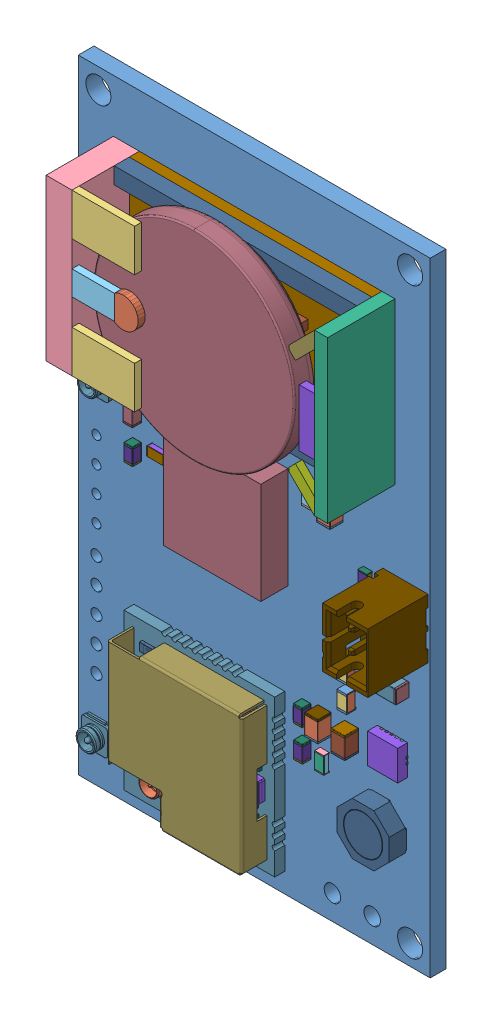
SolidWorks assembly Печатная плата Peggy Tracker, configuration По умолчанию. Lengths in mm.
Overall size (35 62 10.1).
297 component instances, 77 part files, 0 mates.
Components (placement in the parent):
- Печатная плата Peggy Tracker.step-1: Печатная плата Peggy Tracker.step [Default] at origin size (35 62 10.1)
  - Board.step-1: Board.step [Default] at origin size (35 62 1.56)
    - Open CASCADE STEP translator 6.8 1.1.1.step-1: Open CASCADE STEP translator 6.8 1.1.1.step [Default] at (0 0 -1.5596) size (35 62 1.56)
  - X1.step-1: X1.step [Default] at origin size (28 20 6.7)
    - 6517451856.step-1: 6517451856.step [Default] at (11.15 51.75 6) size (3 3 0.7)
      - Extruded.step-1: Extruded.step [Default] at origin size (3 3 0.7)
    - 6517450176.step-1: 6517450176.step [Default] at (9.1815 45.8445 6) size (6.22 4.19 0.7)
      - Extruded-0.step-1: Extruded-0.step [Default] at origin size (6.22 4.19 0.7)
    - 6517450176.step-2: 6517450176.step [Default] at (9.1815 57.6545 6) size (6.22 4.19 0.7)
      - Extruded-0.step-1: Extruded-0.step [Default] at origin size (6.22 4.19 0.7)
    - 6517449536.step-1: 6517449536.step [Default] at (4.785 51.7495 0) size (2.57 16 6.7)
      - Extruded-1.step-1: Extruded-1.step [Default] at origin size (2.57 16 6.7)
    - 6517449376.step-1: 6517449376.step [Default] at (8.1819 51.7635 6) size (4.22 2.41 0.7)
      - Extruded-2.step-1: Extruded-2.step [Default] at origin size (4.22 2.41 0.7)
    - 6517449056.step-1: 6517449056.step [Default] at (30.8492 51.7495 0) size (1.3 16 6.7)
      - Extruded-3.step-1: Extruded-3.step [Default] at origin size (1.3 16 6.7)
    - 6517448576.step-1: 6517448576.step [Default] at (28.9305 45.5257 6) size (2.54 3.55 0.7)
      - Extruded-4.step-1: Extruded-4.step [Default] at origin size (2.54 3.55 0.7)
    - 6517448256.step-1: 6517448256.step [Default] at (29.4382 51.4325 6) size (1.52 5.71 0.7)
      - Extruded-5.step-1: Extruded-5.step [Default] at origin size (1.52 5.71 0.7)
    - 6517447856.step-1: 6517447856.step [Default] at (18.1354 51.7495 0) size (24.13 16 1)
      - Extruded-6.step-1: Extruded-6.step [Default] at origin size (24.13 16 1)
    - 6517447456.step-1: 6517447456.step [Default] at (18.135 58.925 0) size (24.13 1.65 2.5)
      - Extruded-7.step-1: Extruded-7.step [Default] at origin size (24.13 1.65 2.5)
    - 6517447456.step-2: 6517447456.step [Default] at (18.1356 44.5737 0) size (24.13 1.65 2.5)
      - Extruded-7.step-1: Extruded-7.step [Default] at origin size (24.13 1.65 2.5)
    - 6517447056.step-1: 6517447056.step [Default] at (19.0875 48.7663 0) size (9.53 0.89 2.5)
      - Extruded-8.step-1: Extruded-8.step [Default] at origin size (9.53 0.89 2.5)
    - 6517447056.step-2: 6517447056.step [Default] at (19.0875 54.2273 0) size (9.53 0.89 2.5)
      - Extruded-8.step-1: Extruded-8.step [Default] at origin size (9.53 0.89 2.5)
    - 6517446256.step-1: 6517446256.step [Default] at (28.9302 57.972 6) size (2.54 3.55 0.7)
      - Extruded-9.step-1: Extruded-9.step [Default] at origin size (2.54 3.55 0.7)
    - CircuitWorks-BATT_CR2032.step-1: CircuitWorks-BATT_CR2032.step [Default] at (17.5 51.75 6) x (1 0 0) z (0 1 0) size (20 3.2 20)
  - XW2.step-1: XW2.step [Default] at origin size (2.86 3.01 1.29)
    - IPX.step-1: IPX.step [Default] at (2.0669 38.1281 1.27) x (0 1 0) z (0 0 1) size (3.01 2.86 1.29)
  - XW1.step-1: XW1.step [Default] at origin size (2.86 3.01 1.29)
    - IPX.step-1: IPX.step [Default] at (1.9653 7.4677 1.27) x (0 1 0) z (0 0 1) size (3.01 2.86 1.29)
  - R6.step-1: R6.step [Default] at origin size (0.9 1.7 0.55)
    - 6482559680.step-1: 6482559680.step [Default] at (28.8001 34.2999 0) x (0 -1 0) z (0 0 1) size (1.7 0.9 0.55)
      - Terminal.step-1: Terminal.step [Default] at (-0.85 -0.45 0) size (0.1 0.9 0.55)
        - Open_CASCADE_STEP_translator_6.8_15.2.1.step-1: Open_CASCADE_STEP_translator_6.8_15.2.1.step [Default] at origin size (0.1 0.9 0.55)
      - Terminal.step-2: Terminal.step [Default] at (0.85 0.45 0) x (-1 0 0) z (0 0 1) size (0.1 0.9 0.55)
        - Open_CASCADE_STEP_translator_6.8_15.2.1.step-1: Open_CASCADE_STEP_translator_6.8_15.2.1.step [Default] at origin size (0.1 0.9 0.55)
      - Mid_Body.step-1: Mid_Body.step [Default] at (-0.85 -0.45 0) size (1.59 0.9 0.44)
      - Mark.step-1: Mark.step [Default] at (-0.75 -0.45 0.495) size (1.5 0.9 0.06)
  - X3.step-1: X3.step [Default] at origin size (4.5 5.9 9.4)
    - B2B-PH-K-S(LF)(SN)--3DModel-STEP-56544.step-1: B2B-PH-K-S(LF)(SN)--3DModel-STEP-56544.step [Default] at (32.5449 33.0001 3) x (0 -1 0) z (-1 0 0) size (5.9 9.4 4.5)
  - R5.step-1: R5.step [Default] at origin size (0.95 1.75 0.95)
    - 6482560720.step-1: 6482560720.step [Default] at (27.1578 23.3326 0) x (0 1 0) z (0 0 1) size (1.75 0.95 0.95)
      - Terminal-1.step-1: Terminal-1.step [Default] at (-0.875 -0.475 0) size (0.2 0.95 0.95)
        - Open_CASCADE_STEP_translator_6.8_12.2.1.step-1: Open_CASCADE_STEP_translator_6.8_12.2.1.step [Default] at origin size (0.2 0.95 0.95)
      - Terminal-1.step-2: Terminal-1.step [Default] at (0.875 0.475 0) x (-1 0 0) z (0 0 1) size (0.2 0.95 0.95)
        - Open_CASCADE_STEP_translator_6.8_12.2.1.step-1: Open_CASCADE_STEP_translator_6.8_12.2.1.step [Default] at origin size (0.2 0.95 0.95)
      - Mid_Body-10.step-1: Mid_Body-10.step [Default] at (-0.875 -0.475 0) size (1.56 0.95 0.76)
      - Mark-11.step-1: Mark-11.step [Default] at (-0.675 -0.475 0.855) size (1.35 0.95 0.1)
  - R4.step-1: R4.step [Default] at origin size (0.95 1.75 0.95)
    - 6482560720.step-1: 6482560720.step [Default] at (27.1578 25.8726 0) x (0 1 0) z (0 0 1) size (1.75 0.95 0.95)
      - Terminal-1.step-1: Terminal-1.step [Default] at (-0.875 -0.475 0) size (0.2 0.95 0.95)
        - Open_CASCADE_STEP_translator_6.8_12.2.1.step-1: Open_CASCADE_STEP_translator_6.8_12.2.1.step [Default] at origin size (0.2 0.95 0.95)
      - Terminal-1.step-2: Terminal-1.step [Default] at (0.875 0.475 0) x (-1 0 0) z (0 0 1) size (0.2 0.95 0.95)
        - Open_CASCADE_STEP_translator_6.8_12.2.1.step-1: Open_CASCADE_STEP_translator_6.8_12.2.1.step [Default] at origin size (0.2 0.95 0.95)
      - Mid_Body-10.step-1: Mid_Body-10.step [Default] at (-0.875 -0.475 0) size (1.56 0.95 0.76)
      - Mark-11.step-1: Mark-11.step [Default] at (-0.675 -0.475 0.855) size (1.35 0.95 0.1)
  - R3.step-1: R3.step [Default] at origin size (0.9 1.7 0.55)
    - 6482559680.step-1: 6482559680.step [Default] at (28.8001 31.7999 0) x (0 -1 0) z (0 0 1) size (1.7 0.9 0.55)
      - Terminal.step-1: Terminal.step [Default] at (-0.85 -0.45 0) size (0.1 0.9 0.55)
        - Open_CASCADE_STEP_translator_6.8_15.2.1.step-1: Open_CASCADE_STEP_translator_6.8_15.2.1.step [Default] at origin size (0.1 0.9 0.55)
      - Terminal.step-2: Terminal.step [Default] at (0.85 0.45 0) x (-1 0 0) z (0 0 1) size (0.1 0.9 0.55)
        - Open_CASCADE_STEP_translator_6.8_15.2.1.step-1: Open_CASCADE_STEP_translator_6.8_15.2.1.step [Default] at origin size (0.1 0.9 0.55)
      - Mid_Body.step-1: Mid_Body.step [Default] at (-0.85 -0.45 0) size (1.59 0.9 0.44)
      - Mark.step-1: Mark.step [Default] at (-0.75 -0.45 0.495) size (1.5 0.9 0.06)
  - R2.step-1: R2.step [Default] at origin size (0.9 1.7 0.55)
    - 6482559840.step-1: 6482559840.step [Default] at (24.5109 16.5497 0) x (0 1 0) z (0 0 1) size (1.7 0.9 0.55)
      - Terminal-2.step-1: Terminal-2.step [Default] at (-0.85 -0.45 0) size (0.1 0.9 0.55)
        - Open_CASCADE_STEP_translator_6.8_15.2.1-12.step-1: Open_CASCADE_STEP_translator_6.8_15.2.1-12.step [Default] at origin size (0.1 0.9 0.55)
      - Terminal-2.step-2: Terminal-2.step [Default] at (0.85 0.45 0) x (-1 0 0) z (0 0 1) size (0.1 0.9 0.55)
        - Open_CASCADE_STEP_translator_6.8_15.2.1-12.step-1: Open_CASCADE_STEP_translator_6.8_15.2.1-12.step [Default] at origin size (0.1 0.9 0.55)
      - Mid_Body-13.step-1: Mid_Body-13.step [Default] at (-0.85 -0.45 0) size (1.59 0.9 0.44)
      - Mark-14.step-1: Mark-14.step [Default] at (-0.75 -0.45 0.495) size (1.5 0.9 0.06)
  - R1.step-1: R1.step [Default] at origin size (1.7 0.9 0.55)
    - 6517452256.step-1: 6517452256.step [Default] at (8.2043 34.8489 0) size (1.7 0.9 0.55)
      - Terminal-3.step-1: Terminal-3.step [Default] at (-0.85 -0.45 0) size (0.1 0.9 0.55)
        - Open_CASCADE_STEP_translator_6.8_15.2.1-15.step-1: Open_CASCADE_STEP_translator_6.8_15.2.1-15.step [Default] at origin size (0.1 0.9 0.55)
      - Terminal-3.step-2: Terminal-3.step [Default] at (0.85 0.45 0) x (-1 0 0) z (0 0 1) size (0.1 0.9 0.55)
        - Open_CASCADE_STEP_translator_6.8_15.2.1-15.step-1: Open_CASCADE_STEP_translator_6.8_15.2.1-15.step [Default] at origin size (0.1 0.9 0.55)
      - Mid_Body-16.step-1: Mid_Body-16.step [Default] at (-0.85 -0.45 0) size (1.59 0.9 0.44)
      - Mark-17.step-1: Mark-17.step [Default] at (-0.75 -0.45 0.495) size (1.5 0.9 0.06)
  - L2.step-1: L2.step [Default] at origin size (5.2 5.2 1.8)
    - 6482573440.step-1: 6482573440.step [Default] at (30.1268 13.8076 0.2) x (1 0 0) z (0 -1 0) size (5.2 1.8 5.2)
  - L1.step-1: L1.step [Default] at origin size (0.95 1.75 0.95)
    - 6482561680.step-1: 6482561680.step [Default] at (5.85 37.366 0) x (0 1 0) z (0 0 1) size (1.75 0.95 0.95)
      - Terminal-4.step-1: Terminal-4.step [Default] at (-0.875 -0.475 0) size (1.75 0.95 0.95)
        - Open_CASCADE_STEP_translator_6.8_2.1.1.step-1: Open_CASCADE_STEP_translator_6.8_2.1.1.step [Default] at origin size (0.2 0.95 0.95)
        - Open_CASCADE_STEP_translator_6.8_2.1.2.step-1: Open_CASCADE_STEP_translator_6.8_2.1.2.step [Default] at origin size (0.2 0.95 0.95)
      - Mid_Body-18.step-1: Mid_Body-18.step [Default] at (-0.875 -0.475 0) size (1.35 0.95 0.95)
        - Open_CASCADE_STEP_translator_6.8_2.2.1.step-1: Open_CASCADE_STEP_translator_6.8_2.2.1.step [Default] at origin size (1.35 0.95 0.95)
  - DD2.step-1: DD2.step [Default] at origin size (15 15.5 3.52)
    - 3D_RAK3172.step-1: 3D_RAK3172.step [Default] at (20.536 20.4601 1) x (-1 0 0) z (0 0 1) size (15 15.5 3.52)
      - Board-1.step-1: Board-1.step [Default] at origin size (15 15.5 1.01)
        - Open_CASCADE_STEP_translator_6.8_1.1.1.step-1: Open_CASCADE_STEP_translator_6.8_1.1.1.step [Default] at (0 0 -1.014) size (15 15.5 1.01)
          - Open_CASCADE_STEP_translator_6.8_1.1.1.1.step-1: Open_CASCADE_STEP_translator_6.8_1.1.1.1.step [Default] at origin size (15 15.5 1.01)
      - R11.step-1: R11.step [Default] at origin size (0.6 0.3 0.3)
        - 0201_SMD_Capacitor.step-1: 0201_SMD_Capacitor.step [Default] at (3.4751 6.9342 0.2794) x (-1 0 0) z (0 0 1) size (0.6 0.3 0.3)
      - U2.step-1: U2.step [Default] at origin size (0.99 1.02 0.75)
        - 6590464912.step-1: 6590464912.step [Default] at (5.4483 13.05 0) size (0.99 1.02 0.75)
          - Extruded-19.step-1: Extruded-19.step [Default] at origin size (0.99 1.02 0.75)
      - R4-1.step-1: R4-1.step [Default] at origin size (0.68 0.33 0.34)
        - R0201.step-1: R0201.step [Default] at (3.9176 5.9192 0) x (1 0 0) z (0 -1 0) size (0.68 0.34 0.33)
      - R3-1.step-1: R3-1.step [Default] at origin size (0.33 0.68 0.34)
        - R0201.step-1: R0201.step [Default] at (4.1676 5.6692 0) x (0 1 0) z (1 0 0) size (0.68 0.34 0.33)
      - L2-1.step-1: L2-1.step [Default] at origin size (1.15 0.55 0.41)
        - RES_1005-0402.step-1: RES_1005-0402.step [Default] at (2.2661 6.0198 0) x (1 0 0) z (0 -1 0) size (1.15 0.41 0.55)
      - C10.step-1: C10.step [Default] at origin size (0.6 0.3 0.3)
        - 0201_SMD_Capacitor.step-1: 0201_SMD_Capacitor.step [Default] at (7.1835 13.462 0.2794) x (-1 0 0) z (0 0 1) size (0.6 0.3 0.3)
      - C9.step-1: C9.step [Default] at origin size (0.6 0.3 0.3)
        - 0201_SMD_Capacitor.step-1: 0201_SMD_Capacitor.step [Default] at (7.1835 13.97 0.2794) x (-1 0 0) z (0 0 1) size (0.6 0.3 0.3)
      - C8.step-1: C8.step [Default] at origin size (0.6 0.3 0.3)
        - 0201_SMD_Capacitor.step-1: 0201_SMD_Capacitor.step [Default] at (7.1835 12.954 0.2794) x (-1 0 0) z (0 0 1) size (0.6 0.3 0.3)
      - C7.step-1: C7.step [Default] at origin size (0.6 0.3 0.3)
        - 0201_SMD_Capacitor.step-1: 0201_SMD_Capacitor.step [Default] at (6.0793 11.938 0.2794) x (1 0 0) z (0 0 1) size (0.6 0.3 0.3)
      - C6.step-1: C6.step [Default] at origin size (0.6 0.3 0.3)
        - 0201_SMD_Capacitor.step-1: 0201_SMD_Capacitor.step [Default] at (3.8855 13.5541 0.2794) x (-1 0 0) z (0 0 1) size (0.6 0.3 0.3)
      - CON1.step-1: CON1.step [Default] at origin size (3.4 3.1 1.25)
        - UFL-R-SMD.step-1: UFL-R-SMD.step [Default] at (11.3537 12.7757 0) x (1 0 0) z (0 0 1) size (3.4 3.1 1.25)
          - Part_525.step-1: Part_525.step [Default] at origin size (3 2.6 0.35)
          - Part_739.step-1: Part_739.step [Default] at origin size (2 2 0.9)
          - Part_578.step-1: Part_578.step [Default] at origin size (0.6 0.5 0.1)
          - Part_540.step-1: Part_540.step [Default] at origin size (0.4 1.8 0.1)
          - Part_562.step-1: Part_562.step [Default] at origin size (0.4 1.8 0.1)
          - Part_555.step-1: Part_555.step [Default] at origin size (0.6 0.5 0.1)
      - C4.step-1: C4.step [Default] at origin size (0.6 0.3 0.3)
        - 0201_SMD_Capacitor.step-1: 0201_SMD_Capacitor.step [Default] at (3.7799 9.398 0.2794) x (-1 0 0) z (0 0 1) size (0.6 0.3 0.3)
      - U1.step-1: U1.step [Default] at origin size (7.02 7.02 0.8)
        - QFN48_7x7.step-1: QFN48_7x7.step [Default] at (8.8366 6.9818 0) x (0 1 0) z (1 0 0) size (7.02 0.8 7.02)
      - X1-1.step-1: X1-1.step [Default] at origin size (1.61 2.01 0.71)
        - NT2016SA.step-1: NT2016SA.step [Default] at (1.7496 8.4946 0) x (0 1 0) z (1 0 0) size (2.01 0.71 1.61)
      - C43.step-1: C43.step [Default] at origin size (0.6 0.3 0.3)
        - 0201_SMD_Capacitor.step-1: 0201_SMD_Capacitor.step [Default] at (3.7799 9.9822 0.2794) x (-1 0 0) z (0 0 1) size (0.6 0.3 0.3)
      - C42.step-1: C42.step [Default] at origin size (0.3 0.6 0.3)
        - 0201_SMD_Capacitor.step-1: 0201_SMD_Capacitor.step [Default] at (3.0734 7.9709 0.2794) x (0 -1 0) z (0 0 1) size (0.6 0.3 0.3)
      - R9.step-1: R9.step [Default] at origin size (0.6 0.3 0.3)
        - 0201_SMD_Capacitor.step-1: 0201_SMD_Capacitor.step [Default] at (3.7799 8.8138 0.2794) x (-1 0 0) z (0 0 1) size (0.6 0.3 0.3)
      - C1.step-1: C1.step [Default] at origin size (0.6 0.3 0.3)
        - 0201_SMD_Capacitor.step-1: 0201_SMD_Capacitor.step [Default] at (7.0445 11.557 0.2794) x (1 0 0) z (0 0 1) size (0.6 0.3 0.3)
      - C2.step-1: C2.step [Default] at origin size (0.3 0.6 0.3)
        - 0201_SMD_Capacitor.step-1: 0201_SMD_Capacitor.step [Default] at (7.9756 12.2635 0.2794) x (0 -1 0) z (0 0 1) size (0.6 0.3 0.3)
      - C3.step-1: C3.step [Default] at origin size (0.3 0.6 0.3)
        - 0201_SMD_Capacitor.step-1: 0201_SMD_Capacitor.step [Default] at (2.1844 13.4518 0.2794) x (0 -1 0) z (0 0 1) size (0.6 0.3 0.3)
      - C11.step-1: C11.step [Default] at origin size (0.6 0.3 0.3)
        - 0201_SMD_Capacitor.step-1: 0201_SMD_Capacitor.step [Default] at (1.6623 11.9866 0.2794) x (1 0 0) z (0 0 1) size (0.6 0.3 0.3)
      - C12.step-1: C12.step [Default] at origin size (0.6 0.3 0.3)
        - 0201_SMD_Capacitor.step-1: 0201_SMD_Capacitor.step [Default] at (3.2813 12.573 0.2794) x (1 0 0) z (0 0 1) size (0.6 0.3 0.3)
      - C13.step-1: C13.step [Default] at origin size (0.3 0.6 0.3)
        - 0201_SMD_Capacitor.step-1: 0201_SMD_Capacitor.step [Default] at (4.4958 12.0697 0.2794) x (0 1 0) z (0 0 1) size (0.6 0.3 0.3)
      - C14.step-1: C14.step [Default] at origin size (0.3 0.6 0.3)
        - 0201_SMD_Capacitor.step-1: 0201_SMD_Capacitor.step [Default] at (2.7178 12.6739 0.2794) x (0 -1 0) z (0 0 1) size (0.6 0.3 0.3)
      - C17.step-1: C17.step [Default] at origin size (0.3 0.6 0.3)
        - 0201_SMD_Capacitor.step-1: 0201_SMD_Capacitor.step [Default] at (7.6708 14.4693 0.2794) x (0 -1 0) z (0 0 1) size (0.6 0.3 0.3)
      - C18.step-1: C18.step [Default] at origin size (0.6 0.3 0.3)
        - 0201_SMD_Capacitor.step-1: 0201_SMD_Capacitor.step [Default] at (9.1901 14.1224 0.2794) x (-1 0 0) z (0 0 1) size (0.6 0.3 0.3)
      - C19.step-1: C19.step [Default] at origin size (0.3 0.6 0.3)
        - 0201_SMD_Capacitor.step-1: 0201_SMD_Capacitor.step [Default] at (2.8814 10.8799 0.2794) x (0 1 0) z (0 0 1) size (0.6 0.3 0.3)
      - C22.step-1: C22.step [Default] at origin size (0.3 0.6 0.3)
        - 0201_SMD_Capacitor.step-1: 0201_SMD_Capacitor.step [Default] at (2.0432 11.4801 0.2794) x (0 -1 0) z (0 0 1) size (0.6 0.3 0.3)
      - C21.step-1: C21.step [Default] at origin size (0.3 0.6 0.3)
        - 0201_SMD_Capacitor.step-1: 0201_SMD_Capacitor.step [Default] at (1.5606 11.4801 0.2794) x (0 -1 0) z (0 0 1) size (0.6 0.3 0.3)
      - C23.step-1: C23.step [Default] at origin size (1 0.5 0.5)
        - C0402.step-1: C0402.step [Default] at (8.9644 1.5539 0.254) x (1 0 0) z (0 0 1) size (1 0.5 0.5)
      - C24.step-1: C24.step [Default] at origin size (0.6 0.3 0.3)
        - 0201_SMD_Capacitor.step-1: 0201_SMD_Capacitor.step [Default] at (4.7197 3.8862 0.2794) x (-1 0 0) z (0 0 1) size (0.6 0.3 0.3)
      - C26.step-1: C26.step [Default] at origin size (0.3 0.6 0.3)
        - 0201_SMD_Capacitor.step-1: 0201_SMD_Capacitor.step [Default] at (10.541 2.2265 0.2794) x (0 -1 0) z (0 0 1) size (0.6 0.3 0.3)
      - C44.step-1: C44.step [Default] at origin size (0.6 0.3 0.3)
        - 0201_SMD_Capacitor.step-1: 0201_SMD_Capacitor.step [Default] at (4.7919 9.9822 0.2794) x (-1 0 0) z (0 0 1) size (0.6 0.3 0.3)
      - C29.step-1: C29.step [Default] at origin size (0.6 0.3 0.3)
        - 0201_SMD_Capacitor.step-1: 0201_SMD_Capacitor.step [Default] at (3.9925 7.8486 0.2794) x (1 0 0) z (0 0 1) size (0.6 0.3 0.3)
      - C25.step-1: C25.step [Default] at origin size (0.3 0.6 0.3)
        - 0201_SMD_Capacitor.step-1: 0201_SMD_Capacitor.step [Default] at (10.287 1.6263 0.2794) x (0 1 0) z (0 0 1) size (0.6 0.3 0.3)
      - C31.step-1: C31.step [Default] at origin size (0.6 0.3 0.3)
        - 0201_SMD_Capacitor.step-1: 0201_SMD_Capacitor.step [Default] at (3.9965 7.239 0.2794) x (1 0 0) z (0 0 1) size (0.6 0.3 0.3)
      - C32.step-1: C32.step [Default] at origin size (0.6 0.3 0.3)
        - 0201_SMD_Capacitor.step-1: 0201_SMD_Capacitor.step [Default] at (7.8533 2.3622 0.2794) x (1 0 0) z (0 0 1) size (0.6 0.3 0.3)
      - C33.step-1: C33.step [Default] at origin size (1 0.5 0.5)
        - C0402.step-1: C0402.step [Default] at (5.3048 2.0461 0.254) x (-1 0 0) z (0 0 1) size (1 0.5 0.5)
      - C34.step-1: C34.step [Default] at origin size (0.3 0.6 0.3)
        - 0201_SMD_Capacitor.step-1: 0201_SMD_Capacitor.step [Default] at (4.318 4.2211 0.2794) x (0 1 0) z (0 0 1) size (0.6 0.3 0.3)
      - C35.step-1: C35.step [Default] at origin size (0.6 0.3 0.3)
        - 0201_SMD_Capacitor.step-1: 0201_SMD_Capacitor.step [Default] at (9.0365 2.3622 0.2794) x (1 0 0) z (0 0 1) size (0.6 0.3 0.3)
      - C36.step-1: C36.step [Default] at origin size (0.3 0.6 0.3)
        - 0201_SMD_Capacitor.step-1: 0201_SMD_Capacitor.step [Default] at (13.0302 10.0751 0.2794) x (0 -1 0) z (0 0 1) size (0.6 0.3 0.3)
      - C37.step-1: C37.step [Default] at origin size (0.3 0.6 0.3)
        - 0201_SMD_Capacitor.step-1: 0201_SMD_Capacitor.step [Default] at (3.7338 4.2211 0.2794) x (0 1 0) z (0 0 1) size (0.6 0.3 0.3)
      - C38.step-1: C38.step [Default] at origin size (1 0.5 0.5)
        - C0402.step-1: C0402.step [Default] at (2.3114 4.7323 0.254) x (1 0 0) z (0 0 1) size (1 0.5 0.5)
      - C39.step-1: C39.step [Default] at origin size (0.6 0.3 0.3)
        - 0201_SMD_Capacitor.step-1: 0201_SMD_Capacitor.step [Default] at (4.0593 3.1881 0.2794) x (-1 0 0) z (0 0 1) size (0.6 0.3 0.3)
      - C40.step-1: C40.step [Default] at origin size (0.3 0.6 0.3)
        - 0201_SMD_Capacitor.step-1: 0201_SMD_Capacitor.step [Default] at (3.6576 1.7319 0.2794) x (0 1 0) z (0 0 1) size (0.6 0.3 0.3)
      - L1-1.step-1: L1-1.step [Default] at origin size (0.68 0.33 0.34)
        - R0201.step-1: R0201.step [Default] at (7.8526 11.2014 0) x (-1 0 0) z (0 1 0) size (0.68 0.34 0.33)
      - L3.step-1: L3.step [Default] at origin size (0.33 0.68 0.34)
        - R0201.step-1: R0201.step [Default] at (1.7272 13.1318 0) x (0 -1 0) z (-1 0 0) size (0.68 0.34 0.33)
      - L5.step-1: L5.step [Default] at origin size (0.68 0.33 0.34)
        - R0201.step-1: R0201.step [Default] at (8.0772 13.3096 0) x (-1 0 0) z (0 1 0) size (0.68 0.34 0.33)
      - L6.step-1: L6.step [Default] at origin size (1 0.5 0.5)
        - C0402.step-1: C0402.step [Default] at (5.822 11.0823 0.254) x (1 0 0) z (0 0 1) size (1 0.5 0.5)
      - L7.step-1: L7.step [Default] at origin size (0.68 0.33 0.34)
        - R0201.step-1: R0201.step [Default] at (3.5854 12.1158 0) x (1 0 0) z (0 -1 0) size (0.68 0.34 0.33)
      - L9.step-1: L9.step [Default] at origin size (1.15 0.55 0.41)
        - RES_1005-0402.step-1: RES_1005-0402.step [Default] at (3.9641 11.3538 0) x (-1 0 0) z (0 1 0) size (1.15 0.41 0.55)
      - L20.step-1: L20.step [Default] at origin size (1.6 0.8 0.3)
        - 6559637360.step-1: 6559637360.step [Default] at (12.3698 2.0828 0) x (-1 0 0) z (0 1 0) size (1.6 0.3 0.8)
      - L30.step-1: L30.step [Default] at origin size (1.15 0.55 0.41)
        - RES_1005-0402.step-1: RES_1005-0402.step [Default] at (7.1263 1.8 0) x (-1 0 0) z (0 1 0) size (1.15 0.41 0.55)
      - X2.step-1: X2.step [Default] at origin size (1.2 2 0.61)
        - crystal_rtf2012.step-1: crystal_rtf2012.step [Default] at (2.25 2.8402 0) x (0 1 0) z (1 0 0) size (2 0.61 1.2)
      - R2-1.step-1: R2-1.step [Default] at origin size (0.68 0.33 0.34)
        - R0201.step-1: R0201.step [Default] at (1.9613 10.1854 0) x (1 0 0) z (0 -1 0) size (0.68 0.34 0.33)
      - C5.step-1: C5.step [Default] at origin size (0.6 0.3 0.3)
        - 0201_SMD_Capacitor.step-1: 0201_SMD_Capacitor.step [Default] at (1.8749 6.9342 0.2794) x (-1 0 0) z (0 0 1) size (0.6 0.3 0.3)
      - Free-Models.step-1: Free-Models.step [Default] at origin size (13.4 13.9 2.5)
        - D030A-______.step-1: D030A-______.step [Default] at (2.429 -1.8288 0) size (13.4 13.9 2.5)
  - DD1.step-1: DD1.step [Default] at origin size (9.7 10.1 2.8)
    - 6482566000.step-1: 6482566000.step [Default] at (16.1 34.85 0) x (1 0 0) z (0 0 1) size (9.7 10.1 2.8)
      - Body.step-1: Body.step [Default] at (0 0 0.1) size (9.7 10.1 2.7)
      - Pins.step-1: Pins.step [Default] at origin size (9.56 9.36 0.1)
  - DA1.step-1: DA1.step [Default] at origin size (3 3 1)
    - 6482561360.step-1: 6482561360.step [Default] at (31.2728 20.6686 0) x (0 1 0) z (0 0 1) size (3 3 1)
      - FRAME-DRC0010J.step-1: FRAME-DRC0010J.step [Default] x (1 0 0) z (0 -1 0) size (3 0.2 3)
        - Open CASCADE STEP translator 6.8 1.16.1.2.1.step-1: Open CASCADE STEP translator 6.8 1.16.1.2.1.step [Default] at origin size (1.9 0.2 3)
        - Open CASCADE STEP translator 6.8 1.16.1.2.2.step-1: Open CASCADE STEP translator 6.8 1.16.1.2.2.step [Default] at origin size (0.4 0.2 0.24)
        - Open CASCADE STEP translator 6.8 1.16.1.2.3.step-1: Open CASCADE STEP translator 6.8 1.16.1.2.3.step [Default] at origin size (0.4 0.2 0.24)
        - Open CASCADE STEP translator 6.8 1.16.1.2.4.step-1: Open CASCADE STEP translator 6.8 1.16.1.2.4.step [Default] at origin size (0.4 0.2 0.24)
        - Open CASCADE STEP translator 6.8 1.16.1.2.5.step-1: Open CASCADE STEP translator 6.8 1.16.1.2.5.step [Default] at origin size (0.4 0.2 0.24)
        - Open CASCADE STEP translator 6.8 1.16.1.2.6.step-1: Open CASCADE STEP translator 6.8 1.16.1.2.6.step [Default] at origin size (0.4 0.2 0.24)
        - Open CASCADE STEP translator 6.8 1.16.1.2.7.step-1: Open CASCADE STEP translator 6.8 1.16.1.2.7.step [Default] at origin size (0.4 0.2 0.24)
        - Open CASCADE STEP translator 6.8 1.16.1.2.8.step-1: Open CASCADE STEP translator 6.8 1.16.1.2.8.step [Default] at origin size (0.4 0.2 0.24)
        - Open CASCADE STEP translator 6.8 1.16.1.2.9.step-1: Open CASCADE STEP translator 6.8 1.16.1.2.9.step [Default] at origin size (0.4 0.2 0.24)
        - Open CASCADE STEP translator 6.8 1.16.1.2.10.step-1: Open CASCADE STEP translator 6.8 1.16.1.2.10.step [Default] at origin size (0.4 0.2 0.24)
        - Open CASCADE STEP translator 6.8 1.16.1.2.11.step-1: Open CASCADE STEP translator 6.8 1.16.1.2.11.step [Default] at origin size (0.4 0.2 0.24)
      - BODY-SON.step-1: BODY-SON.step [Default] at (0 0 0.025) x (1 0 0) z (0 -1 0) size (3 0.97 3)
  - C8-1.step-1: C8-1.step [Default] at origin size (1.4 2.15 1.4)
    - 6482573680.step-1: 6482573680.step [Default] at (27.1929 19.9035 0) x (0 -1 0) z (0 0 1) size (2.15 1.4 1.4)
      - Terminal-5.step-1: Terminal-5.step [Default] at (-1.075 -0.7 0) size (2.15 1.4 1.4)
        - Open_CASCADE_STEP_translator_6.8_5.1.1.step-1: Open_CASCADE_STEP_translator_6.8_5.1.1.step [Default] at origin size (0.2 1.4 1.4)
        - Open_CASCADE_STEP_translator_6.8_5.1.2.step-1: Open_CASCADE_STEP_translator_6.8_5.1.2.step [Default] at origin size (0.2 1.4 1.4)
      - Mid_Body-1.step-1: Mid_Body-1.step [Default] at (-1.075 -0.7 0) size (1.75 1.4 1.4)
        - Open_CASCADE_STEP_translator_6.8_5.2.1.step-1: Open_CASCADE_STEP_translator_6.8_5.2.1.step [Default] at origin size (1.75 1.4 1.4)
  - C7-1.step-1: C7-1.step [Default] at origin size (2.1 1.35 1.35)
    - 6482573600.step-1: 6482573600.step [Default] at (31.889 26.8 0) x (1 0 0) z (0 0 1) size (2.1 1.35 1.35)
      - Terminal-6.step-1: Terminal-6.step [Default] at (-1.05 -0.675 0) size (2.1 1.35 1.35)
        - Open_CASCADE_STEP_translator_6.8_24.1.1.step-1: Open_CASCADE_STEP_translator_6.8_24.1.1.step [Default] at origin size (0.2 1.35 1.35)
        - Open_CASCADE_STEP_translator_6.8_24.1.2.step-1: Open_CASCADE_STEP_translator_6.8_24.1.2.step [Default] at origin size (0.2 1.35 1.35)
      - Mid_Body-2.step-1: Mid_Body-2.step [Default] at (-1.05 -0.675 0) size (1.7 1.35 1.35)
        - Open_CASCADE_STEP_translator_6.8_24.2.1.step-1: Open_CASCADE_STEP_translator_6.8_24.2.1.step [Default] at origin size (1.7 1.35 1.35)
  - C6-1.step-1: C6-1.step [Default] at origin size (0.9 1.7 0.9)
    - 6482559520.step-1: 6482559520.step [Default] at (22.727 16.763 0) x (0 -1 0) z (0 0 1) size (1.7 0.9 0.9)
      - Terminal-7.step-1: Terminal-7.step [Default] at (-0.85 -0.45 0) size (1.7 0.9 0.9)
        - Open_CASCADE_STEP_translator_6.8_5.1.1-20.step-1: Open_CASCADE_STEP_translator_6.8_5.1.1-20.step [Default] at origin size (0.2 0.9 0.9)
        - Open_CASCADE_STEP_translator_6.8_5.1.2-21.step-1: Open_CASCADE_STEP_translator_6.8_5.1.2-21.step [Default] at origin size (0.2 0.9 0.9)
      - Mid_Body-3.step-1: Mid_Body-3.step [Default] at (-0.85 -0.45 0) size (1.3 0.9 0.9)
        - Open_CASCADE_STEP_translator_6.8_5.2.1-22.step-1: Open_CASCADE_STEP_translator_6.8_5.2.1-22.step [Default] at origin size (1.3 0.9 0.9)
  - C5-1.step-1: C5-1.step [Default] at origin size (1.35 2.1 1.35)
    - 6482568960.step-1: 6482568960.step [Default] at (24.505 19.939 0) x (0 -1 0) z (0 0 1) size (2.1 1.35 1.35)
      - Terminal-8.step-1: Terminal-8.step [Default] at (-1.05 -0.675 0) size (2.1 1.35 1.35)
        - Open_CASCADE_STEP_translator_6.8_24.1.1-23.step-1: Open_CASCADE_STEP_translator_6.8_24.1.1-23.step [Default] at origin size (0.2 1.35 1.35)
        - Open_CASCADE_STEP_translator_6.8_24.1.2-24.step-1: Open_CASCADE_STEP_translator_6.8_24.1.2-24.step [Default] at origin size (0.2 1.35 1.35)
      - Mid_Body-4.step-1: Mid_Body-4.step [Default] at (-1.05 -0.675 0) size (1.7 1.35 1.35)
        - Open_CASCADE_STEP_translator_6.8_24.2.1-25.step-1: Open_CASCADE_STEP_translator_6.8_24.2.1-25.step [Default] at origin size (1.7 1.35 1.35)
  - C4-1.step-1: C4-1.step [Default] at origin size (0.9 1.7 0.9)
    - 6482559520.step-1: 6482559520.step [Default] at (22.7 19.888 0) x (0 -1 0) z (0 0 1) size (1.7 0.9 0.9)
      - Terminal-7.step-1: Terminal-7.step [Default] at (-0.85 -0.45 0) size (1.7 0.9 0.9)
        - Open_CASCADE_STEP_translator_6.8_5.1.1-20.step-1: Open_CASCADE_STEP_translator_6.8_5.1.1-20.step [Default] at origin size (0.2 0.9 0.9)
        - Open_CASCADE_STEP_translator_6.8_5.1.2-21.step-1: Open_CASCADE_STEP_translator_6.8_5.1.2-21.step [Default] at origin size (0.2 0.9 0.9)
      - Mid_Body-3.step-1: Mid_Body-3.step [Default] at (-0.85 -0.45 0) size (1.3 0.9 0.9)
        - Open_CASCADE_STEP_translator_6.8_5.2.1-22.step-1: Open_CASCADE_STEP_translator_6.8_5.2.1-22.step [Default] at origin size (1.3 0.9 0.9)
  - C3-1.step-1: C3-1.step [Default] at origin size (1.35 2.1 1.35)
    - 6482568960.step-1: 6482568960.step [Default] at (25.7048 39.0008 0) x (0 -1 0) z (0 0 1) size (2.1 1.35 1.35)
      - Terminal-8.step-1: Terminal-8.step [Default] at (-1.05 -0.675 0) size (2.1 1.35 1.35)
        - Open_CASCADE_STEP_translator_6.8_24.1.1-23.step-1: Open_CASCADE_STEP_translator_6.8_24.1.1-23.step [Default] at origin size (0.2 1.35 1.35)
        - Open_CASCADE_STEP_translator_6.8_24.1.2-24.step-1: Open_CASCADE_STEP_translator_6.8_24.1.2-24.step [Default] at origin size (0.2 1.35 1.35)
      - Mid_Body-4.step-1: Mid_Body-4.step [Default] at (-1.05 -0.675 0) size (1.7 1.35 1.35)
        - Open_CASCADE_STEP_translator_6.8_24.2.1-25.step-1: Open_CASCADE_STEP_translator_6.8_24.2.1-25.step [Default] at origin size (1.7 1.35 1.35)
  - C2-1.step-1: C2-1.step [Default] at origin size (0.9 1.7 0.9)
    - 6482561200.step-1: 6482561200.step [Default] at (23.5204 39.0508 0) x (0 1 0) z (0 0 1) size (1.7 0.9 0.9)
      - Terminal-9.step-1: Terminal-9.step [Default] at (-0.85 -0.45 0) size (1.7 0.9 0.9)
        - Open_CASCADE_STEP_translator_6.8_5.1.1-26.step-1: Open_CASCADE_STEP_translator_6.8_5.1.1-26.step [Default] at origin size (0.2 0.9 0.9)
        - Open_CASCADE_STEP_translator_6.8_5.1.2-27.step-1: Open_CASCADE_STEP_translator_6.8_5.1.2-27.step [Default] at origin size (0.2 0.9 0.9)
      - Mid_Body-5.step-1: Mid_Body-5.step [Default] at (-0.85 -0.45 0) size (1.3 0.9 0.9)
        - Open_CASCADE_STEP_translator_6.8_5.2.1-28.step-1: Open_CASCADE_STEP_translator_6.8_5.2.1-28.step [Default] at origin size (1.3 0.9 0.9)
  - C1-1.step-1: C1-1.step [Default] at origin size (0.9 1.7 0.9)
    - 6482559520.step-1: 6482559520.step [Default] at (5.842 33.9488 0) x (0 -1 0) z (0 0 1) size (1.7 0.9 0.9)
      - Terminal-7.step-1: Terminal-7.step [Default] at (-0.85 -0.45 0) size (1.7 0.9 0.9)
        - Open_CASCADE_STEP_translator_6.8_5.1.1-20.step-1: Open_CASCADE_STEP_translator_6.8_5.1.1-20.step [Default] at origin size (0.2 0.9 0.9)
        - Open_CASCADE_STEP_translator_6.8_5.1.2-21.step-1: Open_CASCADE_STEP_translator_6.8_5.1.2-21.step [Default] at origin size (0.2 0.9 0.9)
      - Mid_Body-3.step-1: Mid_Body-3.step [Default] at (-0.85 -0.45 0) size (1.3 0.9 0.9)
        - Open_CASCADE_STEP_translator_6.8_5.2.1-22.step-1: Open_CASCADE_STEP_translator_6.8_5.2.1-22.step [Default] at origin size (1.3 0.9 0.9)
